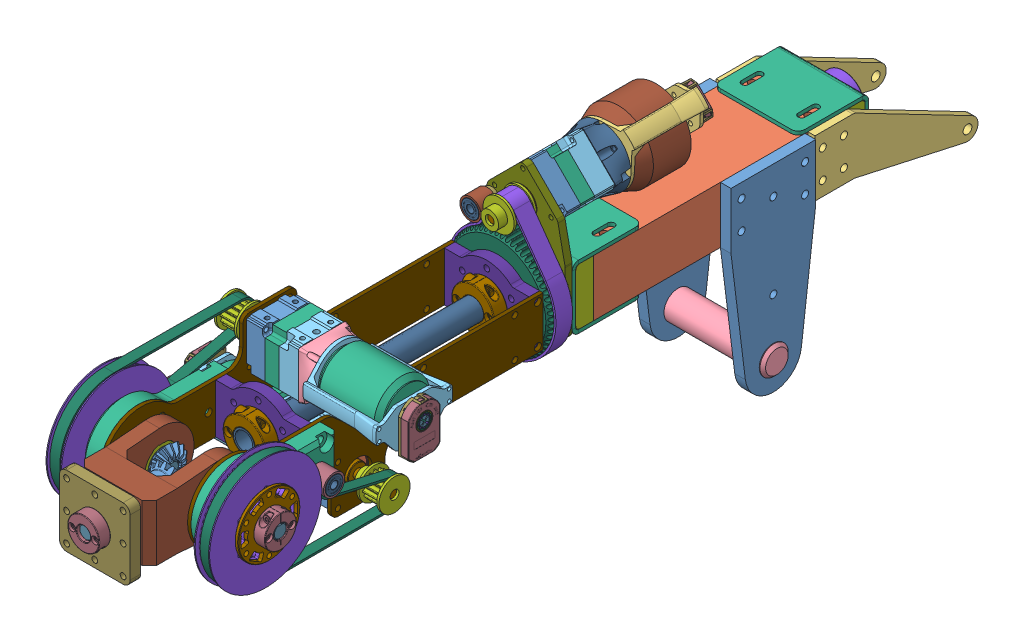
SolidWorks assembly Forearm, configuration Default. Lengths in mm.
Overall size (202.09 263.47 760.46).
240 component instances, 76 part files, 85 mates.
Components (placement in the parent):
- SidePlate^Forearm-1: SidePlate^Forearm [Default] at origin size (9.52 177.8 76.2) (virtual)
- SidePlate^Forearm-2: SidePlate^Forearm [Default] x (-1 0 0) z (0 0 -1) size (9.52 177.8 76.2) (virtual)
- Box^Forearm-1: Box^Forearm [Default] at origin size (76.2 50.8 228.6) (virtual)
- BackSidePlate^Forearm-1: BackSidePlate^Forearm [Default] at origin size (6.35 73.03 146.68) (virtual)
- BackSidePlate^Forearm-2: BackSidePlate^Forearm [Default] at (82.55 0 0) size (6.35 73.03 146.68) (virtual)
- 6061K602_HARDENED PRECISION STEEL SHAFT-1: 6061K602_HARDENED PRECISION STEEL SHAFT [6061K602] at (0 634.475 0) size (101.6 25.4 25.4)
- 6384K367_BALL BEARING-1: 6384K367_BALL BEARING [6384K367] at (0 761.475 166.624) x (1 0 0) z (0 0 -1) size (44.45 44.45 14.3)
- BearingHolder^Forearm-1: BearingHolder^Forearm [Default] at origin size (76.2 57.15 63.5) (virtual)
- BearingSpacer^Forearm-1: BearingSpacer^Forearm [Default] at origin size (76.2 50.8 22.22) (virtual)
- BearingSpacer^Forearm-2: BearingSpacer^Forearm [Default] at (0 0 76.2) x (-1 0 0) z (0 0 -1) size (76.2 50.8 22.22) (virtual)
- BearingHolder^Forearm-2: BearingHolder^Forearm [Default] at (0 0 76.2) x (-1 0 0) z (0 0 -1) size (76.2 57.15 63.5) (virtual)
- 6384K367_BALL BEARING-2: 6384K367_BALL BEARING [6384K367] at (0 761.475 -90.424) x (-1 0 0) z (0 0 1) size (44.45 44.45 14.3)
- 6435K160_ONE-PIECE CLAMP-ON SHAFT COLLAR-1: 6435K160_ONE-PIECE CLAMP-ON SHAFT COLLAR [6435K16] at (0 761.475 -104.7242) x (1 0 0) z (0 0 -1) size (38.1 38.11 12.77)
- 9677T100_CLAMP-ON SHAFT COLLAR WITH MOUNTING HOLES-1: 9677T100_CLAMP-ON SHAFT COLLAR WITH MOUNTING HOLES [9677T1] at (0 761.475 216.6017) x (0 -1 0) z (0 0 -1) size (38.14 38.1 13.27)
- 89955K599_Tube^Forearm-1: 89955K599_Tube^Forearm [Default] at origin size (19.05 19.05 539.7) (virtual)
- ThrustBase^Forearm-1: ThrustBase^Forearm [Default] at origin size (44.45 44.45 14.62) (virtual)
- 5909K460_THRUST NEEDLE-ROLLER BEARING-1: 5909K460_THRUST NEEDLE-ROLLER BEARING [5909K46] at (0 761.475 188.4045) x (0 0 -1) z (1 0 0) size (0.81 31.75 31.75)
- 5909K330_THRUST NEEDLE-ROLLER BEARING-1: 5909K330_THRUST NEEDLE-ROLLER BEARING [5909K33] at (0 761.475 189.3967) x (1 0 0) z (0 1 0) size (31.75 1.98 31.75)
- 5909K460_THRUST NEEDLE-ROLLER BEARING-2: 5909K460_THRUST NEEDLE-ROLLER BEARING [5909K46] at (0 761.475 191.2017) x (0 0 -1) z (1 0 0) size (0.81 31.75 31.75)
- PulleySupportPlate^Forearm-1: PulleySupportPlate^Forearm [Default] at origin size (63.5 63.5 3.18) (virtual)
- J4Pulley-1: J4Pulley [Default] at (0 761.475 197.5517) x (-1 0 0) z (0 -1 0) size (93.75 20.68 93.75)
- J4MotorPlate^Forearm-1: J4MotorPlate^Forearm [Default] at origin size (76.2 120.26 6.35) (virtual)
- WristHub^Forearm-1: WristHub^Forearm [Default] at origin size (76.2 63.5 9.53) (virtual)
- WristSidePlate^Forearm-1: WristSidePlate^Forearm [Default] at origin size (3.17 95.35 628.6) (virtual)
- WristHub^Forearm-2: WristHub^Forearm [Default] at (0 0 205.6733) size (76.2 63.5 9.53) (virtual)
- 9677T100_CLAMP-ON SHAFT COLLAR WITH MOUNTING HOLES-2: 9677T100_CLAMP-ON SHAFT COLLAR WITH MOUNTING HOLES [9677T1] at (0 761.475 422.275) x (0 -1 0) z (0 0 -1) size (38.14 38.1 13.27)
- 6843K130_MTL MITER GEAR--20 DEG PRESSURE ANGLE-1: 6843K130_MTL MITER GEAR--20 DEG PRESSURE ANGLE [6843K13] at (-31.1638 717.333 470.788) x (0 -0.999847 0.017483) z (0 0.017483 0.999847) size (34.68 21.82 34.5)
- 6843K130_MTL MITER GEAR--20 DEG PRESSURE ANGLE-3: 6843K130_MTL MITER GEAR--20 DEG PRESSURE ANGLE [6843K13] at (-11.812 717.333 513.7638) x (0.017483 -0.999847 0) z (0.999847 0.017483 0) size (34.68 21.82 34.5)
- 6384K361_BALL BEARING-1-1: 6384K361_BALL BEARING-1 [6384K361] at (-41.3385 761.475 482.6) x (0 0 1) z (-1 0 0) size (31.75 31.75 11.13)
- 5909K440_THRUST NEEDLE-ROLLER BEARING-1: 5909K440_THRUST NEEDLE-ROLLER BEARING [5909K44] at (-34.5472 761.475 482.6) size (0.81 23.81 23.81)
- 5909K310_THRUST NEEDLE-ROLLER BEARING-1: 5909K310_THRUST NEEDLE-ROLLER BEARING [5909K31] at (-32.7422 761.475 482.6) x (0 1 0) z (0 0 1) size (23.81 1.98 23.81)
- MiterSpacer^Forearm-1: MiterSpacer^Forearm [Default] at origin size (2.03 31.75 31.75) (virtual)
- SidePrintedSupport^Forearm-1: SidePrintedSupport^Forearm [Default] at origin size (15.88 69.85 115.89) (virtual)
- 6384K361_BALL BEARING-1-2: 6384K361_BALL BEARING-1 [6384K361] at (-53.9115 761.475 482.6) x (0 0 1) z (1 0 0) size (31.75 31.75 11.13)
- SidePrintedSupport^Forearm-2: SidePrintedSupport^Forearm [Default] at (0 1522.95 0) x (-1 0 0) z (0 0 1) size (15.88 69.85 115.89) (virtual)
- 6384K361_BALL BEARING-1-3: 6384K361_BALL BEARING-1 [6384K361] at (53.9115 761.475 482.6) x (0 0 -1) z (-1 0 0) size (31.75 31.75 11.13)
- 6384K361_BALL BEARING-1-4: 6384K361_BALL BEARING-1 [6384K361] at (41.3385 761.475 482.6) x (0 0 -1) z (1 0 0) size (31.75 31.75 11.13)
- MiterSpacer^Forearm-2: MiterSpacer^Forearm [Default] at (0 0 965.2) x (-1 0 0) z (0 0 -1) size (2.03 31.75 31.75) (virtual)
- 5909K440_THRUST NEEDLE-ROLLER BEARING-2: 5909K440_THRUST NEEDLE-ROLLER BEARING [5909K44] at (34.5472 761.475 482.6) x (-1 0 0) z (0 0 -1) size (0.81 23.81 23.81)
- 5909K310_THRUST NEEDLE-ROLLER BEARING-2: 5909K310_THRUST NEEDLE-ROLLER BEARING [5909K31] at (32.7422 761.475 482.6) x (0 1 0) z (0 0 1) size (23.81 1.98 23.81)
- 6843K130_MTL MITER GEAR--20 DEG PRESSURE ANGLE-4: 6843K130_MTL MITER GEAR--20 DEG PRESSURE ANGLE [6843K13] at (31.1638 805.1771 469.252) x (0 0.999847 -0.017483) z (0 0.017483 0.999847) size (34.68 21.82 34.5)
- 6391K281_OIL-EMBEDDED SLEEVE BEARING-1: 6391K281_OIL-EMBEDDED SLEEVE BEARING [6391K281] at (-25.8945 761.475 482.6) x (0 0 1) z (-1 0 0) size (31.78 31.78 12.7)
- 6391K281_OIL-EMBEDDED SLEEVE BEARING-2: 6391K281_OIL-EMBEDDED SLEEVE BEARING [6391K281] at (25.8945 761.475 482.6) x (0 0 1) z (-1 0 0) size (31.78 31.78 12.7)
- PulleyHubbed-1: PulleyHubbed [Default] at (-79.0217 761.475 482.6) x (0 0 1) z (-1 0 0) size (101 101 17.18)
  - 60t_x_18mm_Wide_VersaPulley_Kit_HTD_5mm_VersaKeys_217-3200 v2-1: 60t_x_18mm_Wide_VersaPulley_Kit_HTD_5mm_VersaKeys_217-3200 v2 [Default] at origin size (101 101 14)
    - 60t_x_18mm_Wide_VersaPulley_Kit_HTD_5mm_VersaKeys_217-3200 v2.step-1: 60t_x_18mm_Wide_VersaPulley_Kit_HTD_5mm_VersaKeys_217-3200 v2.step [Default] at origin size (101 101 14)
      - 217-3200-001 Rev3.step-1: 217-3200-001 Rev3.step [Default] at (0 0 -7) size (101 101 10.18)
      - 217-3200-001 Rev3.step-2: 217-3200-001 Rev3.step [Default] at (0 0 -17.825) x (-1 0 0) z (0 0 -1) size (101 101 10.18)
  - 1_2_ID_1_8_Keyway_Aluminum_VersaHub_217-2590 v1-1: 1_2_ID_1_8_Keyway_Aluminum_VersaHub_217-2590 v1 [Default] at (0 0 -14.9375) x (0 0 1) z (1 0 0) size (12.7 55.88 55.88)
- SidePulleySpacer^Forearm-1: SidePulleySpacer^Forearm [Default] at origin size (3.81 17.78 17.78) (virtual)
- PulleyHubbed-2: PulleyHubbed [Default] at (79.0217 761.475 482.6) x (0 0 -1) z (1 0 0) size (101 101 17.18)
  - 60t_x_18mm_Wide_VersaPulley_Kit_HTD_5mm_VersaKeys_217-3200 v2-1: 60t_x_18mm_Wide_VersaPulley_Kit_HTD_5mm_VersaKeys_217-3200 v2 [Default] at origin size (101 101 14)
    - 60t_x_18mm_Wide_VersaPulley_Kit_HTD_5mm_VersaKeys_217-3200 v2.step-1: 60t_x_18mm_Wide_VersaPulley_Kit_HTD_5mm_VersaKeys_217-3200 v2.step [Default] at origin size (101 101 14)
      - 217-3200-001 Rev3.step-1: 217-3200-001 Rev3.step [Default] at (0 0 -7) size (101 101 10.18)
      - 217-3200-001 Rev3.step-2: 217-3200-001 Rev3.step [Default] at (0 0 -17.825) x (-1 0 0) z (0 0 -1) size (101 101 10.18)
  - 1_2_ID_1_8_Keyway_Aluminum_VersaHub_217-2590 v1-1: 1_2_ID_1_8_Keyway_Aluminum_VersaHub_217-2590 v1 [Default] at (0 0 -14.9375) x (0 0 1) z (1 0 0) size (12.7 55.88 55.88)
- SidePulleySpacer^Forearm-2: SidePulleySpacer^Forearm [Default] at (0 0 965.2) x (-1 0 0) z (0 0 -1) size (3.81 17.78 17.78) (virtual)
- WristBase^Forearm-3: WristBase^Forearm [Default] at origin size (64.49 57.15 92.08) (virtual)
- 6384K361_BALL BEARING-1-5: 6384K361_BALL BEARING-1 [6384K361] at (0 761.475 523.9385) size (31.75 31.75 11.13)
- MiterSpacer^Forearm-3: MiterSpacer^Forearm [Default] at (-482.6 0 482.6) x (0 0 -1) z (1 0 0) size (2.03 31.75 31.75) (virtual)
- 5909K440_THRUST NEEDLE-ROLLER BEARING-3: 5909K440_THRUST NEEDLE-ROLLER BEARING [5909K44] at (0 761.475 517.1472) x (0 0 -1) z (1 0 0) size (0.81 23.81 23.81)
- 5909K310_THRUST NEEDLE-ROLLER BEARING-3: 5909K310_THRUST NEEDLE-ROLLER BEARING [5909K31] at (0 761.475 515.3422) x (0 1 0) z (-1 0 0) size (23.81 1.98 23.81)
- 6384K361_BALL BEARING-1-6: 6384K361_BALL BEARING-1 [6384K361] at (0 761.475 542.8615) x (1 0 0) z (0 0 -1) size (31.75 31.75 11.13)
- MiterSpacer^Forearm-4: MiterSpacer^Forearm [Default] at (-482.6 0 513.0768) x (0 0 -1) z (1 0 0) size (2.03 31.75 31.75) (virtual)
- 5909K440_THRUST NEEDLE-ROLLER BEARING-4: 5909K440_THRUST NEEDLE-ROLLER BEARING [5909K44] at (0 761.475 550.4656) x (0 0 -1) z (1 0 0) size (0.81 23.81 23.81)
- 5909K440_THRUST NEEDLE-ROLLER BEARING-5: 5909K440_THRUST NEEDLE-ROLLER BEARING [5909K44] at (0 761.475 553.2628) x (0 0 -1) z (1 0 0) size (0.81 23.81 23.81)
- 5909K310_THRUST NEEDLE-ROLLER BEARING-4: 5909K310_THRUST NEEDLE-ROLLER BEARING [5909K31] at (0 761.475 551.4578) x (0 1 0) z (-1 0 0) size (23.81 1.98 23.81)
- HandPlate^Forearm-1: HandPlate^Forearm [Default] at origin size (63.5 63.5 9.52) (virtual)
- 9677T210_CLAMP-ON SHAFT COLLAR WITH MOUNTING HOLES-1: 9677T210_CLAMP-ON SHAFT COLLAR WITH MOUNTING HOLES [9677T21] at (0 761.475 567.9472) x (0 1 0) z (0 0 -1) size (28.6 28.57 10.69)
- 9677T210_CLAMP-ON SHAFT COLLAR WITH MOUNTING HOLES-2: 9677T210_CLAMP-ON SHAFT COLLAR WITH MOUNTING HOLES [9677T21] at (-81.9436 761.475 482.6) x (0 -1 0) z (1 0 0) size (28.6 28.57 10.69)
- 9677T210_CLAMP-ON SHAFT COLLAR WITH MOUNTING HOLES-3: 9677T210_CLAMP-ON SHAFT COLLAR WITH MOUNTING HOLES [9677T21] at (81.9436 761.475 482.6) x (0 -1 0) z (-1 0 0) size (28.6 28.57 10.69)
- 8488T310_FULLY KEYED PRECISION DRIVE SHAFT W CERT-1: 8488T310_FULLY KEYED PRECISION DRIVE SHAFT W CERT [8488T31] at (-48.5172 761.475 482.6) x (0 0 1) z (-1 0 0) size (12.7 12.5 76.2)
- 8488T310_FULLY KEYED PRECISION DRIVE SHAFT W CERT-2: 8488T310_FULLY KEYED PRECISION DRIVE SHAFT W CERT [8488T31] at (48.5172 761.475 482.6) x (0 0 1) z (-1 0 0) size (12.7 12.5 76.2)
- 8488T310_FULLY KEYED PRECISION DRIVE SHAFT W CERT-3: 8488T310_FULLY KEYED PRECISION DRIVE SHAFT W CERT [8488T31] at (0 761.475 532.819) size (12.7 12.5 76.2)
- Keda9to1-1: Keda9to1 [Default] at (15.7154 807.3546 154.825) x (0 0 1) z (-0.707107 -0.707107 0) size (176.96 63 76.93)
  - VersaPlanetary_v2_Single_Stage_10_1_with_BAG.STEP-1: VersaPlanetary_v2_Single_Stage_10_1_with_BAG.STEP [Default] at origin size (163.4 63.52 63.52)
    - 217-2820 Rev1_Public.STEP-1: 217-2820 Rev1_Public.STEP [Default] at (-4.6546 22.225 0) x (0 -0.456494 0.889726) z (-1 0 0) size (39.22 38.88 17.4)
      - 217-2625-100.STEP-1: 217-2625-100.STEP [Default] at origin size (39.22 38.88 12.7)
        - 217-2625-008 Rev1.STEP-1: 217-2625-008 Rev1.STEP [Default] at origin size (34.7 34.7 4.7)
        - 217-2625-010 Rev1.STEP-1: 217-2625-010 Rev1.STEP [Default] at (0 10.193 3.65) x (0.999813 0.019336 0) z (0 0 1) size (4 4 12)
        - 217-2625-010 Rev1.STEP-2: 217-2625-010 Rev1.STEP [Default] at (8.691 -5.3258 3.65) size (4 4 12)
        - 217-2625-010 Rev1.STEP-3: 217-2625-010 Rev1.STEP [Default] at (-8.691 -5.3258 3.65) size (4 4 12)
        - 217-2625-005 Rev1_Planet_Revolving_Follower01.STEP-1: 217-2625-005 Rev1_Planet_Revolving_Follower01.STEP [Default] at (8.691 -5.3258 6.35) x (0.932816 0.360354 0) z (0 0 1) size (16.89 16.89 8)
        - 217-2625-005 Rev1_Planet_Revolving_Follower01.STEP-2: 217-2625-005 Rev1_Planet_Revolving_Follower01.STEP [Default] at (-8.691 -5.3258 6.35) x (-0.932788 -0.360426 0) z (0 0 1) size (16.89 16.89 8)
        - 217-2625-005 Rev1_Planet_Revolving_Follower01.STEP-3: 217-2625-005 Rev1_Planet_Revolving_Follower01.STEP [Default] at (0 10.193 6.35) x (0.893583 0.448898 0) z (0 0 1) size (16.89 16.89 8)
      - 217-2625-007 Rev1_Public.STEP-1: 217-2625-007 Rev1_Public.STEP [Default] at (0 0 6.7) x (0.992772 0.120019 0) z (0 0 1) size (15.27 15.27 12.7)
    - 217-2625-026 Rev1.STEP-1: 217-2625-026 Rev1.STEP [Default] at (-6.5 22.225 0) x (0 -1 0) z (-1 0 0) size (44.45 42 18.12)
    - 217-2742-001 Rev4.STEP-1: 217-2742-001 Rev4.STEP [Default] at (0.2002 22.225 0) x (1 0 0) z (0 -0.092627 0.995701) size (7 28 28)
    - 217-2742-001 Rev4.STEP-2: 217-2742-001 Rev4.STEP [Default] at (8.2002 22.225 0) size (7 28 28)
    - 217-2625-017 Rev1_9714K61.STEP-1: 217-2625-017 Rev1_9714K61.STEP [Default] at (7.42 22.3002 -0.342) x (0 0.56703 0.823697) z (0 -0.823697 0.56703) size (28.51 4.98 27.43)
    - 217-2625-003 Rev1.STEP-1: 217-2625-003 Rev1.STEP [Default] at (7.4478 22.225 0) x (0 -1 0) z (1 0 0) size (17 17 64.11) (hidden)
    - 217-2625-018 Rev1_98541A410.STEP-1: 217-2625-018 Rev1_98541A410.STEP [Default] at (-0.7046 22.225 0) x (1 0 0) z (0 -0.017452 0.999848) size (1 19.6 17.4)
    - 832-1750-Ring-Gear-Screw_SSA0832-0500ZC.STEP-1: 832-1750-Ring-Gear-Screw_SSA0832-0500ZC.STEP [Default] at (-30.7 4.725 -17.5) x (0 0.997447 0.071411) z (0 -0.071411 0.997447) size (6.73 48.51 6.73) (hidden)
    - 832-1750-Ring-Gear-Screw_SSA0832-0500ZC.STEP-2: 832-1750-Ring-Gear-Screw_SSA0832-0500ZC.STEP [Default] at (-30.7 39.725 17.5) x (0 0.005929 0.999982) z (0 -0.999982 0.005929) size (6.73 48.51 6.73) (hidden)
    - 217-2625-025 Rev1.STEP-1: 217-2625-025 Rev1.STEP [Default] at (-23.2 22.225 0) x (0 -1 0) z (-1 0 0) size (44.45 42 18)
    - 217-4649-002 Rev1_SSA0832-0500ZC.STEP-1: 217-4649-002 Rev1_SSA0832-0500ZC.STEP [Default] at (-33.7 4.2645 17.9605) x (0 0.33842 -0.940995) z (0 0.940995 0.33842) size (6.73 16.76 6.73) (hidden)
    - 217-4649-002 Rev1_SSA0832-0500ZC.STEP-2: 217-4649-002 Rev1_SSA0832-0500ZC.STEP [Default] at (-33.7 40.1855 -17.9605) x (0 -0.308932 -0.951084) z (0 0.951084 -0.308932) size (6.73 16.76 6.73) (hidden)
    - 217-4649-006 Rev1_SSA0004-008BA.STEP-1: 217-4649-006 Rev1_SSA0004-008BA.STEP [Default] at (-30.7 22.225 12.5) x (0 0.5 -0.866025) z (0 -0.866025 -0.5) size (7 14 7) (hidden)
    - 217-4649-006 Rev1_SSA0004-008BA.STEP-2: 217-4649-006 Rev1_SSA0004-008BA.STEP [Default] at (-30.7 22.225 -12.5) x (0 -0.5 0.866025) z (0 0.866025 0.5) size (7 14 7) (hidden)
    - 217-2822-003 Rev4.STEP-1: 217-2822-003 Rev4.STEP [Default] at (-32.2 22.225 0) x (0 -1 0) z (-1 0 0) size (42 42 4.8) (hidden)
    - 217-3351 Rev2.STEP-1: 217-3351 Rev2.STEP [Default] at (-33.7 22.225 0) x (0 0 1) z (1 0 0) size (59.07 59.07 84.5) (hidden)
    - 217-2816-001 Rev1.STEP-1: 217-2816-001 Rev1.STEP [Default] at (-6.35 22.225 0) x (0 -1 0) z (1 0 0) size (42 42 14.51)
    - 217-4649-001 Rev1.STEP-1: 217-4649-001 Rev1.STEP [Default] at (-20.046 22.225 0) x (0 -1 0) z (1 0 0) size (18 18 13)
    - 217-4649-007 Rev1_94105A824.STEP-1: 217-4649-007 Rev1_94105A824.STEP [Default] at (-25.521 22.225 -6.7835) x (-0.996104 -0.088191 0) z (0 0 -1) size (4.83 4.83 4.77)
    - 217-2625-011 Rev1.STEP-1: 217-2625-011 Rev1.STEP [Default] at (-24.7818 22.225 0) x (0 0 1) z (0 -1 0) size (8.01 7.5 7.94) (hidden)
  - VersaPlanetary_CIM_Motor_Output_Shaft_Kit_217-2893-1: VersaPlanetary_CIM_Motor_Output_Shaft_Kit_217-2893 [Default] at (7.4478 22.225 0) x (0 0 -1) z (1 0 0) size (17 17 57.85)
  - KedaAdapter^Keda9to1-1: KedaAdapter^Keda9to1 [Default] at origin size (17.82 53.01 53.01) (virtual)
  - 192kvMotorEncoded-1: 192kvMotorEncoded [Default] at (-51.0318 22.225 0) x (0 -1 0) z (0 0 -1) size (63 104.52 76.93)
    - BetterKEDA-1: BetterKEDA [Default] at origin size (63 104.52 63)
    - CUI_DEVICES_AMT102-0048-N2000-S-1: CUI_DEVICES_AMT102-0048-N2000-S [Default] at (0 65.12 0) x (1 0 0) z (0 1 0) size (36.33 46.21 9.2)
      - CUI_DEVICES_AMT102-0048-N2000-S.step-1: CUI_DEVICES_AMT102-0048-N2000-S.step [Default] at origin size (36.33 46.21 9.2)
        - AMT-102-Base-REV-K.step-1: AMT-102-Base-REV-K.step [Default] x (-1 0 0) z (0 0 -1) size (28.78 43.39 9.06)
        - AMT-102-Top-Cover-REV-H.step-1: AMT-102-Top-Cover-REV-H.step [Default] at (0 0 5.23) x (-1 0 0) z (0 0 -1) size (28.6 43.26 6.55)
        - AMT-Sleeve-REV-D_ 2 mm.step-1: AMT-Sleeve-REV-D_ 2 mm.step [Default] at (0 0 -2.42) x (0.999996 0.002864 0) z (0 0 1) size (10.79 10.79 7.8)
        - AMT-Hub-Top-REV-D1.step-1: AMT-Hub-Top-REV-D1.step [Default] at (0 0 2.13) x (0.999996 0.002864 0) z (0 0 1) size (14 14 5.67)
        - AMT-Hub-Bottom-REV-B.step-1: AMT-Hub-Bottom-REV-B.step [Default] at (0 0 2.43) x (0.999998 -0.001942 0) z (0 0 1) size (17.3 17.3 3.2)
        - AMT10X-Shaft-Adaptor-REV-E.step-1: AMT10X-Shaft-Adaptor-REV-E.step [Default] at (0 0 0.03) x (0.999996 0.002864 0) z (0 0 1) size (11.8 11.8 7.8)
        - Receiver-board.step-1: Receiver-board.step [Default] at (72.2834 -20.351 3.03) x (-1 0 0) z (0 0 -1) size (26.5 26.62 0.41)
        - Rotor-board-REV F.step-1: Rotor-board-REV F.step [Default] at (0 0 2.13) x (0.807874 -0.589355 0) z (0 0 1) size (26 26 0.3)
        - Transmitter-board AMT10_AMT-102.step-1: Transmitter-board AMT10_AMT-102.step [Default] at (19.1596 -17.1102 1.22) x (-1 0 0) z (0 0 -1) size (26.63 38.43 4.41)
    - Body^192kvMotorEncoded-1: Body^192kvMotorEncoded [Default] at origin size (53 64.53 76.93) (virtual)
- PropDrive10to1-2: PropDrive10to1 [Default] at (-21.475 819.123 367.2673) x (-1 0 0) z (0 0 1) size (173.44 53.05 69.17)
  - VersaPlanetary_v2_Single_Stage_10_1_with_BAG.STEP-1: VersaPlanetary_v2_Single_Stage_10_1_with_BAG.STEP [Default] at origin size (163.4 63.52 63.52)
    - 217-2820 Rev1_Public.STEP-1: 217-2820 Rev1_Public.STEP [Default] at (-4.6546 22.225 0) x (0 -0.456494 0.889726) z (-1 0 0) size (39.22 38.88 17.4)
      - 217-2625-100.STEP-1: 217-2625-100.STEP [Default] at origin size (39.22 38.88 12.7)
        - 217-2625-008 Rev1.STEP-1: 217-2625-008 Rev1.STEP [Default] at origin size (34.7 34.7 4.7)
        - 217-2625-010 Rev1.STEP-1: 217-2625-010 Rev1.STEP [Default] at (0 10.193 3.65) x (0.999813 0.019336 0) z (0 0 1) size (4 4 12)
        - 217-2625-010 Rev1.STEP-2: 217-2625-010 Rev1.STEP [Default] at (8.691 -5.3258 3.65) size (4 4 12)
        - 217-2625-010 Rev1.STEP-3: 217-2625-010 Rev1.STEP [Default] at (-8.691 -5.3258 3.65) size (4 4 12)
        - 217-2625-005 Rev1_Planet_Revolving_Follower01.STEP-1: 217-2625-005 Rev1_Planet_Revolving_Follower01.STEP [Default] at (8.691 -5.3258 6.35) x (0.932816 0.360354 0) z (0 0 1) size (16.89 16.89 8)
        - 217-2625-005 Rev1_Planet_Revolving_Follower01.STEP-2: 217-2625-005 Rev1_Planet_Revolving_Follower01.STEP [Default] at (-8.691 -5.3258 6.35) x (-0.932788 -0.360426 0) z (0 0 1) size (16.89 16.89 8)
        - 217-2625-005 Rev1_Planet_Revolving_Follower01.STEP-3: 217-2625-005 Rev1_Planet_Revolving_Follower01.STEP [Default] at (0 10.193 6.35) x (0.893583 0.448898 0) z (0 0 1) size (16.89 16.89 8)
      - 217-2625-007 Rev1_Public.STEP-1: 217-2625-007 Rev1_Public.STEP [Default] at (0 0 6.7) x (0.992772 0.120019 0) z (0 0 1) size (15.27 15.27 12.7)
    - 217-2625-026 Rev1.STEP-1: 217-2625-026 Rev1.STEP [Default] at (-6.5 22.225 0) x (0 -1 0) z (-1 0 0) size (44.45 42 18.12)
    - 217-2742-001 Rev4.STEP-1: 217-2742-001 Rev4.STEP [Default] at (0.2002 22.225 0) x (1 0 0) z (0 -0.092627 0.995701) size (7 28 28)
    - 217-2742-001 Rev4.STEP-2: 217-2742-001 Rev4.STEP [Default] at (8.2002 22.225 0) size (7 28 28)
    - 217-2625-017 Rev1_9714K61.STEP-1: 217-2625-017 Rev1_9714K61.STEP [Default] at (7.42 22.3002 -0.342) x (0 0.56703 0.823697) z (0 -0.823697 0.56703) size (28.51 4.98 27.43)
    - 217-2625-003 Rev1.STEP-1: 217-2625-003 Rev1.STEP [Default] at (7.4478 22.225 0) x (0 -1 0) z (1 0 0) size (17 17 64.11) (hidden)
    - 217-2625-018 Rev1_98541A410.STEP-1: 217-2625-018 Rev1_98541A410.STEP [Default] at (-0.7046 22.225 0) x (1 0 0) z (0 -0.017452 0.999848) size (1 19.6 17.4)
    - 832-1750-Ring-Gear-Screw_SSA0832-0500ZC.STEP-1: 832-1750-Ring-Gear-Screw_SSA0832-0500ZC.STEP [Default] at (-30.7 4.725 -17.5) x (0 0.997447 0.071411) z (0 -0.071411 0.997447) size (6.73 48.51 6.73) (hidden)
    - 832-1750-Ring-Gear-Screw_SSA0832-0500ZC.STEP-2: 832-1750-Ring-Gear-Screw_SSA0832-0500ZC.STEP [Default] at (-30.7 39.725 17.5) x (0 0.005929 0.999982) z (0 -0.999982 0.005929) size (6.73 48.51 6.73) (hidden)
    - 217-2625-025 Rev1.STEP-1: 217-2625-025 Rev1.STEP [Default] at (-23.2 22.225 0) x (0 -1 0) z (-1 0 0) size (44.45 42 18)
    - 217-4649-002 Rev1_SSA0832-0500ZC.STEP-1: 217-4649-002 Rev1_SSA0832-0500ZC.STEP [Default] at (-33.7 4.2645 17.9605) x (0 0.33842 -0.940995) z (0 0.940995 0.33842) size (6.73 16.76 6.73) (hidden)
    - 217-4649-002 Rev1_SSA0832-0500ZC.STEP-2: 217-4649-002 Rev1_SSA0832-0500ZC.STEP [Default] at (-33.7 40.1855 -17.9605) x (0 -0.308932 -0.951084) z (0 0.951084 -0.308932) size (6.73 16.76 6.73) (hidden)
    - 217-4649-006 Rev1_SSA0004-008BA.STEP-1: 217-4649-006 Rev1_SSA0004-008BA.STEP [Default] at (-30.7 22.225 12.5) x (0 0.5 -0.866025) z (0 -0.866025 -0.5) size (7 14 7) (hidden)
    - 217-4649-006 Rev1_SSA0004-008BA.STEP-2: 217-4649-006 Rev1_SSA0004-008BA.STEP [Default] at (-30.7 22.225 -12.5) x (0 -0.5 0.866025) z (0 0.866025 0.5) size (7 14 7) (hidden)
    - 217-2822-003 Rev4.STEP-1: 217-2822-003 Rev4.STEP [Default] at (-32.2 22.225 0) x (0 -1 0) z (-1 0 0) size (42 42 4.8) (hidden)
    - 217-3351 Rev2.STEP-1: 217-3351 Rev2.STEP [Default] at (-33.7 22.225 0) x (0 0 1) z (1 0 0) size (59.07 59.07 84.5) (hidden)
    - 217-2816-001 Rev1.STEP-1: 217-2816-001 Rev1.STEP [Default] at (-6.35 22.225 0) x (0 -1 0) z (1 0 0) size (42 42 14.51)
    - 217-4649-001 Rev1.STEP-1: 217-4649-001 Rev1.STEP [Default] at (-20.046 22.225 0) x (0 -1 0) z (1 0 0) size (18 18 13)
    - 217-4649-007 Rev1_94105A824.STEP-1: 217-4649-007 Rev1_94105A824.STEP [Default] at (-25.521 22.225 -6.7835) x (-0.996104 -0.088191 0) z (0 0 -1) size (4.83 4.83 4.77)
    - 217-2625-011 Rev1.STEP-1: 217-2625-011 Rev1.STEP [Default] at (-24.7818 22.225 0) x (0 0 1) z (0 -1 0) size (8.01 7.5 7.94) (hidden)
  - VersaPlanetary_CIM_Motor_Output_Shaft_Kit_217-2893-1: VersaPlanetary_CIM_Motor_Output_Shaft_Kit_217-2893 [Default] at (7.4478 22.225 0) x (0 0 -1) z (1 0 0) size (17 17 57.85)
  - PDAdapter^PropDrive10to1-1: PDAdapter^PropDrive10to1 [Default] at origin size (14.63 50.01 50.01) (virtual)
  - 380kvMotorEncoded-1: 380kvMotorEncoded [Default] at (-48.0193 22.225 0) x (0 -1 0) z (0 0 -1) size (53.05 100.5 69.17)
    - CUI_DEVICES_AMT102-0048-N2000-S-1: CUI_DEVICES_AMT102-0048-N2000-S [Default] at (0 69.12 0) x (0 0 1) z (0 1 0) size (36.33 46.21 9.2)
      - CUI_DEVICES_AMT102-0048-N2000-S.step-1: CUI_DEVICES_AMT102-0048-N2000-S.step [Default] at origin size (36.33 46.21 9.2)
        - AMT-102-Base-REV-K.step-1: AMT-102-Base-REV-K.step [Default] x (-1 0 0) z (0 0 -1) size (28.78 43.39 9.06)
        - AMT-102-Top-Cover-REV-H.step-1: AMT-102-Top-Cover-REV-H.step [Default] at (0 0 5.23) x (-1 0 0) z (0 0 -1) size (28.6 43.26 6.55)
        - AMT-Sleeve-REV-D_ 2 mm.step-1: AMT-Sleeve-REV-D_ 2 mm.step [Default] at (0 0 -2.42) x (0.999996 0.002864 0) z (0 0 1) size (10.79 10.79 7.8)
        - AMT-Hub-Top-REV-D1.step-1: AMT-Hub-Top-REV-D1.step [Default] at (0 0 2.13) x (0.999996 0.002864 0) z (0 0 1) size (14 14 5.67)
        - AMT-Hub-Bottom-REV-B.step-1: AMT-Hub-Bottom-REV-B.step [Default] at (0 0 2.43) x (0.999998 -0.001942 0) z (0 0 1) size (17.3 17.3 3.2)
        - AMT10X-Shaft-Adaptor-REV-E.step-1: AMT10X-Shaft-Adaptor-REV-E.step [Default] at (0 0 0.03) x (0.999996 0.002864 0) z (0 0 1) size (11.8 11.8 7.8)
        - Receiver-board.step-1: Receiver-board.step [Default] at (72.2834 -20.351 3.03) x (-1 0 0) z (0 0 -1) size (26.5 26.62 0.41)
        - Rotor-board-REV F.step-1: Rotor-board-REV F.step [Default] at (0 0 2.13) x (0.807874 -0.589355 0) z (0 0 1) size (26 26 0.3)
        - Transmitter-board AMT10_AMT-102.step-1: Transmitter-board AMT10_AMT-102.step [Default] at (19.1596 -17.1102 1.22) x (-1 0 0) z (0 0 -1) size (26.63 38.43 4.41)
    - Body^380kvMotorEncoded-1: Body^380kvMotorEncoded [Default] at origin size (50 68.53 69.17) (virtual)
    - PROPDRIVE v2 5060 380KV Brushless Outrunner Motor-1: PROPDRIVE v2 5060 380KV Brushless Outrunner Motor [Default] x (1 0 0) z (0 0 -1) size (50 100 50)
- WristSidePlate^Forearm-3: WristSidePlate^Forearm [Default] at (0 1522.95 0) x (-1 0 0) z (0 0 1) size (3.17 95.35 628.6) (virtual)
- PropDrive10to1-4: PropDrive10to1 [Default] at (21.475 703.827 367.2673) size (173.44 53.05 69.17)
  - VersaPlanetary_v2_Single_Stage_10_1_with_BAG.STEP-1: VersaPlanetary_v2_Single_Stage_10_1_with_BAG.STEP [Default] at origin size (163.4 63.52 63.52)
    - 217-2820 Rev1_Public.STEP-1: 217-2820 Rev1_Public.STEP [Default] at (-4.6546 22.225 0) x (0 -0.456494 0.889726) z (-1 0 0) size (39.22 38.88 17.4)
      - 217-2625-100.STEP-1: 217-2625-100.STEP [Default] at origin size (39.22 38.88 12.7)
        - 217-2625-008 Rev1.STEP-1: 217-2625-008 Rev1.STEP [Default] at origin size (34.7 34.7 4.7)
        - 217-2625-010 Rev1.STEP-1: 217-2625-010 Rev1.STEP [Default] at (0 10.193 3.65) x (0.999813 0.019336 0) z (0 0 1) size (4 4 12)
        - 217-2625-010 Rev1.STEP-2: 217-2625-010 Rev1.STEP [Default] at (8.691 -5.3258 3.65) size (4 4 12)
        - 217-2625-010 Rev1.STEP-3: 217-2625-010 Rev1.STEP [Default] at (-8.691 -5.3258 3.65) size (4 4 12)
        - 217-2625-005 Rev1_Planet_Revolving_Follower01.STEP-1: 217-2625-005 Rev1_Planet_Revolving_Follower01.STEP [Default] at (8.691 -5.3258 6.35) x (0.932816 0.360354 0) z (0 0 1) size (16.89 16.89 8)
        - 217-2625-005 Rev1_Planet_Revolving_Follower01.STEP-2: 217-2625-005 Rev1_Planet_Revolving_Follower01.STEP [Default] at (-8.691 -5.3258 6.35) x (-0.932788 -0.360426 0) z (0 0 1) size (16.89 16.89 8)
        - 217-2625-005 Rev1_Planet_Revolving_Follower01.STEP-3: 217-2625-005 Rev1_Planet_Revolving_Follower01.STEP [Default] at (0 10.193 6.35) x (0.893583 0.448898 0) z (0 0 1) size (16.89 16.89 8)
      - 217-2625-007 Rev1_Public.STEP-1: 217-2625-007 Rev1_Public.STEP [Default] at (0 0 6.7) x (0.992772 0.120019 0) z (0 0 1) size (15.27 15.27 12.7)
    - 217-2625-026 Rev1.STEP-1: 217-2625-026 Rev1.STEP [Default] at (-6.5 22.225 0) x (0 -1 0) z (-1 0 0) size (44.45 42 18.12)
    - 217-2742-001 Rev4.STEP-1: 217-2742-001 Rev4.STEP [Default] at (0.2002 22.225 0) x (1 0 0) z (0 -0.092627 0.995701) size (7 28 28)
    - 217-2742-001 Rev4.STEP-2: 217-2742-001 Rev4.STEP [Default] at (8.2002 22.225 0) size (7 28 28)
    - 217-2625-017 Rev1_9714K61.STEP-1: 217-2625-017 Rev1_9714K61.STEP [Default] at (7.42 22.3002 -0.342) x (0 0.56703 0.823697) z (0 -0.823697 0.56703) size (28.51 4.98 27.43)
    - 217-2625-003 Rev1.STEP-1: 217-2625-003 Rev1.STEP [Default] at (7.4478 22.225 0) x (0 -1 0) z (1 0 0) size (17 17 64.11) (hidden)
    - 217-2625-018 Rev1_98541A410.STEP-1: 217-2625-018 Rev1_98541A410.STEP [Default] at (-0.7046 22.225 0) x (1 0 0) z (0 -0.017452 0.999848) size (1 19.6 17.4)
    - 832-1750-Ring-Gear-Screw_SSA0832-0500ZC.STEP-1: 832-1750-Ring-Gear-Screw_SSA0832-0500ZC.STEP [Default] at (-30.7 4.725 -17.5) x (0 0.997447 0.071411) z (0 -0.071411 0.997447) size (6.73 48.51 6.73) (hidden)
    - 832-1750-Ring-Gear-Screw_SSA0832-0500ZC.STEP-2: 832-1750-Ring-Gear-Screw_SSA0832-0500ZC.STEP [Default] at (-30.7 39.725 17.5) x (0 0.005929 0.999982) z (0 -0.999982 0.005929) size (6.73 48.51 6.73) (hidden)
    - 217-2625-025 Rev1.STEP-1: 217-2625-025 Rev1.STEP [Default] at (-23.2 22.225 0) x (0 -1 0) z (-1 0 0) size (44.45 42 18)
    - 217-4649-002 Rev1_SSA0832-0500ZC.STEP-1: 217-4649-002 Rev1_SSA0832-0500ZC.STEP [Default] at (-33.7 4.2645 17.9605) x (0 0.33842 -0.940995) z (0 0.940995 0.33842) size (6.73 16.76 6.73) (hidden)
    - 217-4649-002 Rev1_SSA0832-0500ZC.STEP-2: 217-4649-002 Rev1_SSA0832-0500ZC.STEP [Default] at (-33.7 40.1855 -17.9605) x (0 -0.308932 -0.951084) z (0 0.951084 -0.308932) size (6.73 16.76 6.73) (hidden)
    - 217-4649-006 Rev1_SSA0004-008BA.STEP-1: 217-4649-006 Rev1_SSA0004-008BA.STEP [Default] at (-30.7 22.225 12.5) x (0 0.5 -0.866025) z (0 -0.866025 -0.5) size (7 14 7) (hidden)
    - 217-4649-006 Rev1_SSA0004-008BA.STEP-2: 217-4649-006 Rev1_SSA0004-008BA.STEP [Default] at (-30.7 22.225 -12.5) x (0 -0.5 0.866025) z (0 0.866025 0.5) size (7 14 7) (hidden)
    - 217-2822-003 Rev4.STEP-1: 217-2822-003 Rev4.STEP [Default] at (-32.2 22.225 0) x (0 -1 0) z (-1 0 0) size (42 42 4.8) (hidden)
    - 217-3351 Rev2.STEP-1: 217-3351 Rev2.STEP [Default] at (-33.7 22.225 0) x (0 0 1) z (1 0 0) size (59.07 59.07 84.5) (hidden)
    - 217-2816-001 Rev1.STEP-1: 217-2816-001 Rev1.STEP [Default] at (-6.35 22.225 0) x (0 -1 0) z (1 0 0) size (42 42 14.51)
    - 217-4649-001 Rev1.STEP-1: 217-4649-001 Rev1.STEP [Default] at (-20.046 22.225 0) x (0 -1 0) z (1 0 0) size (18 18 13)
    - 217-4649-007 Rev1_94105A824.STEP-1: 217-4649-007 Rev1_94105A824.STEP [Default] at (-25.521 22.225 -6.7835) x (-0.996104 -0.088191 0) z (0 0 -1) size (4.83 4.83 4.77)
    - 217-2625-011 Rev1.STEP-1: 217-2625-011 Rev1.STEP [Default] at (-24.7818 22.225 0) x (0 0 1) z (0 -1 0) size (8.01 7.5 7.94) (hidden)
  - VersaPlanetary_CIM_Motor_Output_Shaft_Kit_217-2893-1: VersaPlanetary_CIM_Motor_Output_Shaft_Kit_217-2893 [Default] at (7.4478 22.225 0) x (0 0 -1) z (1 0 0) size (17 17 57.85)
  - PDAdapter^PropDrive10to1-1: PDAdapter^PropDrive10to1 [Default] at origin size (14.63 50.01 50.01) (virtual)
  - 380kvMotorEncoded-1: 380kvMotorEncoded [Default] at (-48.0193 22.225 0) x (0 -1 0) z (0 0 -1) size (53.05 100.5 69.17)
    - CUI_DEVICES_AMT102-0048-N2000-S-1: CUI_DEVICES_AMT102-0048-N2000-S [Default] at (0 69.12 0) x (0 0 1) z (0 1 0) size (36.33 46.21 9.2)
      - CUI_DEVICES_AMT102-0048-N2000-S.step-1: CUI_DEVICES_AMT102-0048-N2000-S.step [Default] at origin size (36.33 46.21 9.2)
        - AMT-102-Base-REV-K.step-1: AMT-102-Base-REV-K.step [Default] x (-1 0 0) z (0 0 -1) size (28.78 43.39 9.06)
        - AMT-102-Top-Cover-REV-H.step-1: AMT-102-Top-Cover-REV-H.step [Default] at (0 0 5.23) x (-1 0 0) z (0 0 -1) size (28.6 43.26 6.55)
        - AMT-Sleeve-REV-D_ 2 mm.step-1: AMT-Sleeve-REV-D_ 2 mm.step [Default] at (0 0 -2.42) x (0.999996 0.002864 0) z (0 0 1) size (10.79 10.79 7.8)
        - AMT-Hub-Top-REV-D1.step-1: AMT-Hub-Top-REV-D1.step [Default] at (0 0 2.13) x (0.999996 0.002864 0) z (0 0 1) size (14 14 5.67)
        - AMT-Hub-Bottom-REV-B.step-1: AMT-Hub-Bottom-REV-B.step [Default] at (0 0 2.43) x (0.999998 -0.001942 0) z (0 0 1) size (17.3 17.3 3.2)
        - AMT10X-Shaft-Adaptor-REV-E.step-1: AMT10X-Shaft-Adaptor-REV-E.step [Default] at (0 0 0.03) x (0.999996 0.002864 0) z (0 0 1) size (11.8 11.8 7.8)
        - Receiver-board.step-1: Receiver-board.step [Default] at (72.2834 -20.351 3.03) x (-1 0 0) z (0 0 -1) size (26.5 26.62 0.41)
        - Rotor-board-REV F.step-1: Rotor-board-REV F.step [Default] at (0 0 2.13) x (0.807874 -0.589355 0) z (0 0 1) size (26 26 0.3)
        - Transmitter-board AMT10_AMT-102.step-1: Transmitter-board AMT10_AMT-102.step [Default] at (19.1596 -17.1102 1.22) x (-1 0 0) z (0 0 -1) size (26.63 38.43 4.41)
    - Body^380kvMotorEncoded-1: Body^380kvMotorEncoded [Default] at origin size (50 68.53 69.17) (virtual)
    - PROPDRIVE v2 5060 380KV Brushless Outrunner Motor-1: PROPDRIVE v2 5060 380KV Brushless Outrunner Motor [Default] x (1 0 0) z (0 0 -1) size (50 100 50)
